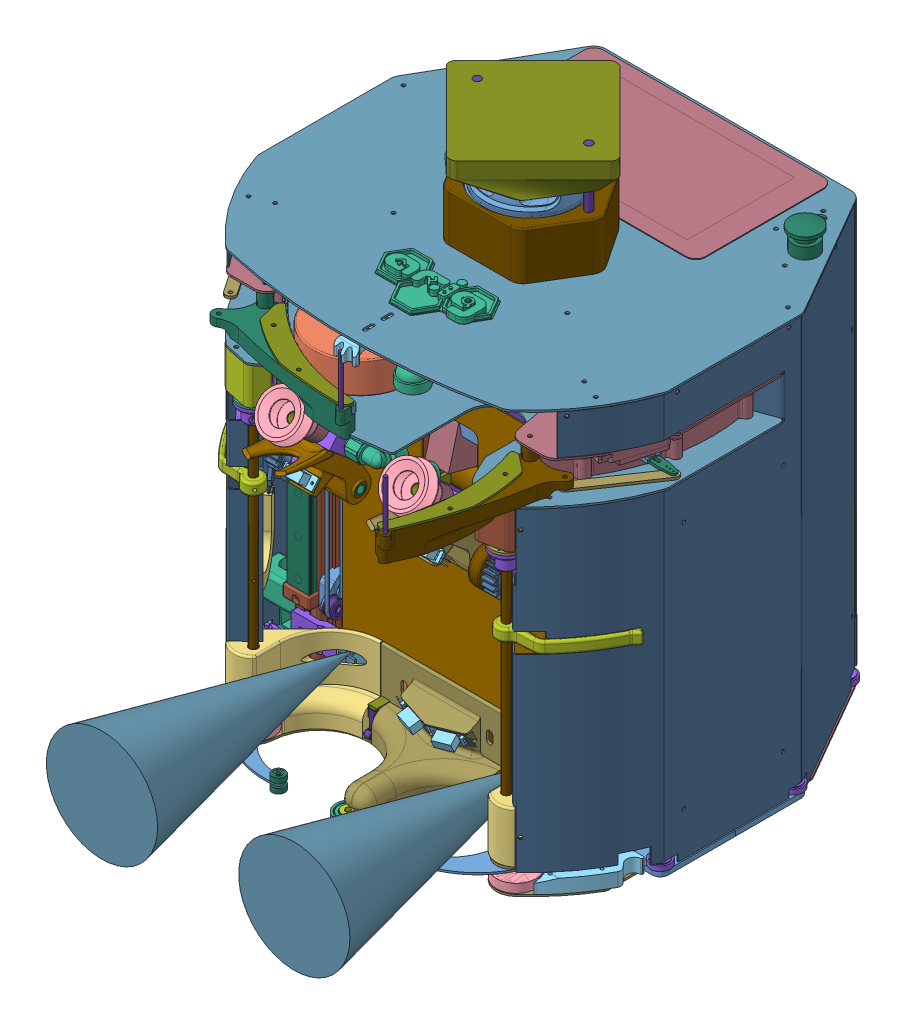
SolidWorks assembly 2019_Gros_robot, configuration Défaut. Lengths in mm.
Overall size (437.04 440.65 488.1).
582 component instances, 188 part files, 267 mates.
Components (placement in the parent):
- Robot2017_BaseRoulante-1: Robot2017_BaseRoulante [Défaut] at origin size (333 188.15 128.41)
  - Robot2015_BaseRoulante_piece01-1: Robot2015_BaseRoulante_piece01 [Défaut] at (0 7 0) size (330 4 120)
  - Robot2015_BaseRoulante_piece02-1: Robot2015_BaseRoulante_piece02 [Défaut] at (88 31 0) size (9.5 55 70)
  - Robot2015_BaseRoulante_piece02-2: Robot2015_BaseRoulante_piece02 [Défaut] at (55 31 0) x (-1 0 0) z (0 0 -1) size (9.5 55 70)
  - Robot2015_BaseRoulante_piece02-3: Robot2015_BaseRoulante_piece02 [Défaut] at (-55 31 0) size (9.5 55 70)
  - Robot2015_BaseRoulante_piece02-4: Robot2015_BaseRoulante_piece02 [Défaut] at (-88 31 0) x (-1 0 0) z (0 0 -1) size (9.5 55 70)
  - RoueMotrice-1: RoueMotrice [Défaut] at (109 -484.4772 -22.3565) x (0 -1 0) z (1 0 0) size (68.64 68.64 30)
    - Pneu-1: Pneu [Défaut] at (-515.4772 -22.3565 -15) size (64 64 30)
    - Jante-1: Jante [Défaut] at (-515.4772 -22.3565 15) x (-0.856398 -0.516316 0) z (0 0 1) size (50 50 30)
  - RoueMotrice-2: RoueMotrice [Défaut] at (-109 178.4325 494.4494) x (0 0.243951 0.969787) z (-1 0 0) size (68.64 68.64 30)
    - Pneu-1: Pneu [Défaut] at (-515.4772 -22.3565 -15) size (64 64 30)
    - Jante-1: Jante [Défaut] at (-515.4772 -22.3565 15) x (-0.856398 -0.516316 0) z (0 0 1) size (50 50 30)
  - Robot2015_BaseRoulante_piece03-1: Robot2015_BaseRoulante_piece03 [Défaut] at (117 31 0) size (67.5 12 14.69)
  - Robot2015_BaseRoulante_piece03-2: Robot2015_BaseRoulante_piece03 [Défaut] at (-117 31 0) x (-1 0 0) z (0 -0.777778 -0.62854) size (67.5 12 14.69)
  - roulement-1: roulement [Défaut] at (90 31 0) size (7 22 22)
  - roulement-2: roulement [Défaut] at (53 31 0) x (1 0 0) z (0 0.679013 0.734126) size (7 22 22)
  - roulement-3: roulement [Défaut] at (-53 31 0) x (1 0 0) z (0 0.679013 0.734126) size (7 22 22)
  - roulement-4: roulement [Défaut] at (-90 31 0) x (1 0 0) z (0 0.679013 0.734126) size (7 22 22)
  - Pignon XL037 pas5.08-1: Pignon XL037 pas5.08 [20 dents] at (67.65 31 0) x (1 0 0) z (0 -0.960015 0.27995) size (22 38 38)
  - Pignon XL037 pas5.08-2: Pignon XL037 pas5.08 [20 dents] at (67.65 149.9855 -19) x (-1 0 0) z (0 0.08811 -0.996111) size (22 38 38)
  - Robot2015_roulementAngle-1: Robot2015_roulementAngle [Défaut] at (158.5 13.75 53.5) size (16 9.5 16)
  - Robot2015_roulementAngle-2: Robot2015_roulementAngle [Défaut] at (158.5 13.75 -53.5) size (16 9.5 16)
  - Robot2015_roulementAngle-3: Robot2015_roulementAngle [Défaut] at (-158.5 13.75 53.5) size (16 9.5 16)
  - Robot2015_roulementAngle-4: Robot2015_roulementAngle [Défaut] at (-158.5 13.75 -53.5) size (16 9.5 16)
  - moteur-1: moteur [Défaut] at (48 149.9855 -19) x (0 -0.99965 -0.026437) z (1 0 0) size (42 42 188.5)
  - moteur-2: moteur [Défaut] at (-48 104.7937 -19) x (0 0.767621 0.640905) z (-1 0 0) size (42 42 188.5)
  - Pignon XL037 pas5.08-3: Pignon XL037 pas5.08 [20 dents] at (-67.65 31 0) x (-1 0 0) z (0 -0.781685 -0.623674) size (22 38 38)
  - Pignon XL037 pas5.08-4: Pignon XL037 pas5.08 [20 dents] at (-67.65 104.7937 -19) x (1 0 0) z (0 0.006752 0.999977) size (22 38 38)
  - Robot2015_profiléX20_01-1: Robot2015_profiléX20_01 [Défaut] at (-28 11 -40) x (0 0 -1) z (0 1 0) size (20 20 165)
  - Robot2015_profiléX20_01-2: Robot2015_profiléX20_01 [Défaut] at (48 11 -40) x (0 0 -1) z (0 1 0) size (20 20 165)
  - Robot2015_BaseRoulante_piece04-1: Robot2015_BaseRoulante_piece04 [Défaut] at (48 149.9855 -58) x (1 0 0) z (0 0 -1) size (3 50 44)
  - Robot2015_BaseRoulante_piece04-2: Robot2015_BaseRoulante_piece04 [Défaut] at (-51 104.7937 -58) x (1 0 0) z (0 0 -1) size (3 50 44)
  - Courroie1-5^Robot2017_BaseRoulante-1: Courroie1-5^Robot2017_BaseRoulante [Défaut] at (-67.65 104.7937 -19) x (0 0 -1) z (1 0 0) size (53.34 108.13 10) (virtual)
  - Courroie2-6^Robot2017_BaseRoulante-1: Courroie2-6^Robot2017_BaseRoulante [Défaut] at (67.65 149.9855 -19) x (0 0 1) z (-1 0 0) size (79.34 153.33 10) (virtual)
  - Robot2015_BaseRoulante_piece06-1: Robot2015_BaseRoulante_piece06 [Défaut] at (0 177.5 -61.5) size (256 20 20)
  - Igus_TK_04_09_Rail_L50-1: Igus_TK_04_09_Rail_L50 [Défaut] at (136 38.5 35) x (0 0 -1) z (1 0 0) size (9.6 50 6.3)
  - Igus_TK_04_09_coulisseau-1: Igus_TK_04_09_coulisseau [Défaut] at (136 101 35) x (0 0 -1) z (1 0 0) size (20 29 8.3)
  - Igus_TK_04_09_Rail_L50-2: Igus_TK_04_09_Rail_L50 [Défaut] at (136 38.5 -35) x (0 0 -1) z (1 0 0) size (9.6 50 6.3)
  - Igus_TK_04_09_coulisseau-2: Igus_TK_04_09_coulisseau [Défaut] at (136 101 -35) x (0 0 -1) z (1 0 0) size (20 29 8.3)
  - Igus_TK_04_09_Rail_L50-3: Igus_TK_04_09_Rail_L50 [Défaut] at (-136 38.5 35) x (0 0 1) z (-1 0 0) size (9.6 50 6.3)
  - Igus_TK_04_09_coulisseau-3: Igus_TK_04_09_coulisseau [Défaut] at (-136 101 35) x (0 0 1) z (-1 0 0) size (20 29 8.3)
  - Igus_TK_04_09_Rail_L50-4: Igus_TK_04_09_Rail_L50 [Défaut] at (-136 38.5 -35) x (0 0 1) z (-1 0 0) size (9.6 50 6.3)
  - Igus_TK_04_09_coulisseau-4: Igus_TK_04_09_coulisseau [Défaut] at (-136 101 -35) x (0 0 1) z (-1 0 0) size (20 29 8.3)
  - Kubler-05.2400.1212.1024-1: Kubler-05.2400.1212.1024 [fil a Gch] at (157 24 0) x (-1 0 0) z (0 0.34202 0.939693) size (31 88.25 62)
    - Kubler-05.2400.1212.1024-1: Kubler-05.2400.1212.1024 [Défaut] at origin size (31 36 24)
    - Kubler-rayon mini cable-1: Kubler-rayon mini cable [Défaut] at (25 -24 0) x (0 0 1) z (-1 0 0) size (52.25 52.25 4.5)
  - Kubler-05.2400.1212.1024-2: Kubler-05.2400.1212.1024 [fil a Drt] at (-157 24 0) x (1 0 0) z (0 -0.34202 -0.939693) size (31 88.25 62)
    - Kubler-05.2400.1212.1024-1: Kubler-05.2400.1212.1024 [Défaut] at origin size (31 36 24)
    - Kubler-rayon mini cable-1: Kubler-rayon mini cable [Défaut] at (25 -24 0) x (0 0 -1) z (1 0 0) size (52.25 52.25 4.5)
  - Robot2015_BaseRoulante_piece07-1: Robot2015_BaseRoulante_piece07 [Défaut] at (146 56.5 0) x (0 0 -1) z (1 0 0) size (93 50 1.5)
  - Robot2015_BaseRoulante_piece07-2: Robot2015_BaseRoulante_piece07 [Défaut] at (-146 56.5 0) x (0 0 1) z (-1 0 0) size (93 50 1.5)
  - Robot2015_BaseRoulante_piece08-1: Robot2015_BaseRoulante_piece08 [Défaut] at (51 38.5 30) size (85 55 10)
  - Robot2015_BaseRoulante_piece09-1: Robot2015_BaseRoulante_piece09 [Défaut] at (51 38.5 -30) x (1 0 0) z (0 0 -1) size (57 55 10)
  - Robot2015_BaseRoulante_piece09-2: Robot2015_BaseRoulante_piece09 [Défaut] at (-51 38.5 -30) x (-1 0 0) z (0 0 -1) size (57 55 10)
  - Robot2015_BaseRoulante_piece08-2: Robot2015_BaseRoulante_piece08 [Défaut] at (-51 38.5 30) x (-1 0 0) z (0 0 1) size (85 55 10)
  - Robot2015_BaseRoulante_piece10-1: Robot2015_BaseRoulante_piece10 [Défaut] at (155 24 0) x (-1 0 0) z (0 -0.545932 -0.837829) size (9 48 48)
  - Robot2015_BaseRoulante_piece10-2: Robot2015_BaseRoulante_piece10 [Défaut] at (-155 24 0) size (9 48 48)
  - Robot2015_BaseRoulante_piece11-1: Robot2015_BaseRoulante_piece11 [Défaut] at (79 66 0) x (0 0 -1) z (1 0 0) size (80 1.5 63)
  - Robot2015_BaseRoulante_piece11-2: Robot2015_BaseRoulante_piece11 [Défaut] at (-79 66 0) x (0 0 1) z (-1 0 0) size (80 1.5 63)
  - Robot2015_BaseRoulante_piece12-1: Robot2015_BaseRoulante_piece12 [Défaut] at (162 11 40) x (-1 0 0) z (0 0 -1) size (11.5 11.5 80)
  - Robot2015_BaseRoulante_piece12-2: Robot2015_BaseRoulante_piece12 [Défaut] at (-162 11 -40) size (11.5 11.5 80)
  - pignon renvoi 20 dents XL 2006-1: pignon renvoi 20 dents XL 2006 [Défaut] at (67.65 40 -45) x (1 0 0) z (0 0.474564 0.880221) size (9 32.34 32.34)
  - 20170402-1131-1: 20170402-1131 [Défaut] at (48 40 -45) x (0 0 -1) z (1 0 0) size (25 50 24.65)
  - 20170402-1229-1: 20170402-1229 [Défaut] at (73.15 40 -38.5) x (0 0 -1) z (1 0 0) size (25.5 30 9)
- batterieLIPO-1: batterieLIPO [Défaut] at (-65 97 -76) size (160 49 34)
- Robot2019_profiléX20_02-1: Robot2019_profiléX20_02 [Défaut] at (-110 276 40) x (0 0 1) z (0 -1 0) size (20 20 265)
- Robot2019_profiléX20_02-2: Robot2019_profiléX20_02 [Défaut] at (-110 276 -60) x (0 0 1) z (0 -1 0) size (20 20 265)
- Robot2019_profiléX20_02-3: Robot2019_profiléX20_02 [Défaut] at (130 276 40) x (0 0 1) z (0 -1 0) size (20 20 265)
- Robot2019_profiléX20_02-4: Robot2019_profiléX20_02 [Défaut] at (130 276 -60) x (0 0 1) z (0 -1 0) size (20 20 265)
- Robot2019_plaque bille porteuseAvant-1: Robot2019_plaque bille porteuseAvant [Défaut] at (0 5.5 0) size (300 1.5 120)
- Robot2019_plaque bille porteuse Arriere-1: Robot2019_plaque bille porteuse Arriere [Défaut] at (0 5.5 0) x (-1 0 0) z (0 0 -1) size (310 1.5 125)
- Robot2019_plaque du dessus-1: Robot2019_plaque du dessus [Défaut] at (0 276 0) size (330 1.5 300.96)
- APEM_A01ES_A0154B-1: APEM_A01ES_A0154B [Défaut] at (121.8383 345 -100) x (0.5 0 0.866025) z (-0.866025 0 0.5) size (24 61 24)
- bille porteuse-3: bille porteuse [Défaut] at (-111.446 0 -110) x (-0.5 0 -0.866025) z (0.866025 0 -0.5) size (49.64 21.5 47.15)
  - Robot2015_support bille porteuse-1: Robot2015_support bille porteuse [Défaut] at (0 9.5 0) size (49.64 12 45)
  - BillePorteuse-1: BillePorteuse [Défaut] at (0 7.5 0) x (0.947171 0 0.32073) z (0.32073 0 -0.947171) size (31 21.5 31)
- bille porteuse-4: bille porteuse [Défaut] at (111.446 0 -110) size (49.64 21.5 47.15)
  - Robot2015_support bille porteuse-1: Robot2015_support bille porteuse [Défaut] at (0 9.5 0) size (49.64 12 45)
  - BillePorteuse-1: BillePorteuse [Défaut] at (0 7.5 0) x (0.947171 0 0.32073) z (0.32073 0 -0.947171) size (31 21.5 31)
- pompe air 12v SFE-1: pompe air 12v SFE [Défaut] at (-20.6394 32 -38) size (38 60 92)
- rplidar-a2-1: rplidar-a2 [Défaut] at (-75 354.2861 -6.0269) x (0 0 -1) z (1 0 0) size (80.61 40.81 84.84)
- Robot2015_roulementAngle-1: Robot2015_roulementAngle [Défaut] at (100.765 9.75 -153.5) size (16 9.5 16)
- Robot2015_roulementAngle-2: Robot2015_roulementAngle [Défaut] at (-100.765 9.75 -153.5) size (16 9.5 16)
- 20180929-0119-1: 20180929-0119 [Défaut] at (0 277.5 0) x (-1 0 0) z (0 0 -1) size (291.8 157.5 260.35) (flexible)
  - Palet-1: Palet [Redium] at (-99.9974 12.7 0.7186) size (76.2 25.4 76.2)
  - Palet-2: Palet [Greenium] at (-49.3764 12.7 86.9596) size (76.2 25.4 76.2)
  - Palet-3: Palet [Redium] at (50.6211 12.7 86.241) size (76.2 25.4 76.2) (hidden)
  - Palet-4: Palet [Blueium] at (99.9974 12.7 -0.7186) x (0.648467 0 0.761243) z (-0.761243 0 0.648467) size (76.2 25.4 76.2)
  - Palet-5: Palet [Greenium] at (49.3764 12.7 -86.9596) x (0.321702 0 0.946841) z (-0.946841 0 0.321702) size (76.2 25.4 76.2)
  - Palet-6: Palet [Redium] at (-50.6211 12.7 -86.241) size (76.2 25.4 76.2) (hidden)
  - roulement-1: roulement [Défaut] at (81.9289 14.5 -48.09) x (0 -1 0) z (0.925744 0 -0.37815) size (7 22 22)
  - roulement-2: roulement [Défaut] at (-0.6827 14.5 -94.9975) x (0 -1 0) z (0.135385 0 -0.990793) size (7 22 22)
  - roulement-3: roulement [Défaut] at (-82.6116 14.5 -46.9075) x (0 -1 0) z (-0.79036 0 -0.612643) size (7 22 22)
  - roulement-4: roulement [Défaut] at (-81.9289 14.5 48.09) x (0 -1 0) z (-0.925744 0 0.37815) size (7 22 22)
  - roulement-5: roulement [Défaut] at (0.6827 14.5 94.9975) x (0 -1 0) z (-0.135385 0 0.990793) size (7 22 22)
  - roulement-6: roulement [Défaut] at (82.6116 14.5 46.9075) x (0 -1 0) z (0.79036 0 0.612643) size (7 22 22)
  - 20190528-1730-1: 20190528-1730 [Défaut] at (0 8.5 -22.5) x (0.926307 0 0.37677) z (-0.37677 0 0.926307) size (29.93 18 29.98)
  - 20181010-0239-1: 20181010-0239 [Défaut] at (0 8.5 0) x (0.853252 0 -0.521498) z (0.521498 0 0.853252) size (122.02 20.9 126.29)
  - PlaqueTounanteCarre94mm-1: PlaqueTounanteCarre94mm [Défaut] x (-0.707107 0 0.707107) z (-0.707107 0 -0.707107) size (115.6 8.5 115.6) (flexible)
    - PlaqueTounanteCarre94mm-1: PlaqueTounanteCarre94mm [Défaut] at origin size (94 8.25 94)
    - PlaqueTounanteCarre94mm-2: PlaqueTounanteCarre94mm [Défaut] at (0 8.5 0) x (-0.265754 0 -0.964041) z (-0.964041 0 0.265754) size (94 8.25 94)
  - 20190123-2151-1: 20190123-2151 [Défaut] at (0 16.5 0) x (-0.506211 0 -0.86241) z (0.86241 0 -0.506211) size (41.57 20.66 45)
  - 20190123-2208-1: 20190123-2208 [Défaut] at (81.9289 17.9 -48.09) x (-0.274765 0 -0.961511) z (-0.961511 0 0.274765) size (11.85 7.9 11.85)
  - 20190123-2208-2: 20190123-2208 [Défaut] at (-0.6827 17.9 -94.9975) x (-0.970076 0 -0.242802) z (-0.242802 0 0.970076) size (11.85 7.9 11.85)
  - 20190123-2208-3: 20190123-2208 [Défaut] at (-82.6116 17.9 -46.9075) x (-0.695311 0 0.718709) z (0.718709 0 0.695311) size (11.85 7.9 11.85)
  - 20190123-2208-4: 20190123-2208 [Défaut] at (-81.9289 17.9 48.09) x (0.274765 0 0.961511) z (0.961511 0 -0.274765) size (11.85 7.9 11.85)
  - 20190123-2208-5: 20190123-2208 [Défaut] at (0.6827 17.9 94.9975) x (0.970076 0 0.242802) z (0.242802 0 -0.970076) size (11.85 7.9 11.85)
  - 20190123-2208-6: 20190123-2208 [Défaut] at (82.6116 17.9 46.9075) x (0.695311 0 -0.718709) z (-0.718709 0 -0.695311) size (11.85 7.9 11.85)
  - 20190123-2151-2: 20190123-2151 [Défaut] at (0 16.5 0) x (-0.999974 0 0.007186) z (-0.007186 0 -0.999974) size (41.57 20.66 45)
  - 20190123-2151-3: 20190123-2151 [Défaut] at (0 16.5 0) x (-0.493764 0 0.869596) z (-0.869596 0 -0.493764) size (41.57 20.66 45)
  - 20190123-2151-4: 20190123-2151 [Défaut] at (0 16.5 0) x (0.506211 0 0.86241) z (-0.86241 0 0.506211) size (41.57 20.66 45)
  - 20190123-2151-5: 20190123-2151 [Défaut] at (0 16.5 0) x (0.999974 0 -0.007186) z (0.007186 0 0.999974) size (41.57 20.66 45)
  - 20190123-2151-6: 20190123-2151 [Défaut] at (0 16.5 0) x (0.493764 0 -0.869596) z (0.869596 0 0.493764) size (41.57 20.66 45)
  - 12v-silent-dc-motor-146rpm-encoder-desc-dime-1: 12v-silent-dc-motor-146rpm-encoder-desc-dime [Défaut] at (0 -2.5 -22.5) x (0 -1 0) z (-0.707107 0 -0.707107) size (123 36 36)
  - 20190124-0048-1: 20190124-0048 [Défaut] at (0 26.5 -22.5) x (0.37677 0 -0.926307) z (0.926307 0 0.37677) size (15 43 15)
  - NBB1,5-F79-E0-1: NBB1,5-F79-E0 [Défaut] at (43 30 0) x (1 0 0) z (0 0 -1) size (21 4.7 8)
  - 20190124-0123-1: 20190124-0123 [Défaut] at (47 32 -6.05) x (0 0 1) z (-1 0 0) size (19 4 16)
- 20181001-1750-1: 20181001-1750 [Défaut] at origin size (319.23 251.89 229.82)
  - Access_HS-645_BrasRondPetitModele-2: Access_HS-645_BrasRondPetitModele [Défaut] at (94 221.9292 85.221) x (0 0.153259 -0.988186) z (0 0.988186 0.153259) size (24 5 24)
  - Palet-1: Palet [Redium] at (50 270.0402 158.1056) x (1 0 0) z (0 0.766044 -0.642788) size (76.2 25.4 76.2) (hidden)
  - Servo_HS-805-BB-1: Servo_HS-805-BB [Défaut] at (-29 228 9) x (0 0.965926 -0.258819) z (0 0.258819 0.965926) size (82 65 29.5)
  - Access_HS-805_BrasRond-1: Access_HS-805_BrasRond [Défaut] at (-89 228 9) x (0 0 -1) z (0 1 0) size (39.6 8.5 39.6)
  - HIWIN_MGW09H 1 R 200 ZF H M SS_FILE-1: HIWIN_MGW09H 1 R 200 ZF H M SS_FILE [Défaut] at (-120 68 60) size (18 200 7)
  - HIWIN_MGW09H 1 R 200 ZF H M SS_FILE_1-1: HIWIN_MGW09H 1 R 200 ZF H M SS_FILE_1 [Défaut] at (-120 181.8091 60) size (30 51.3 9.1)
  - HIWIN_MGW09H 1 R 200 ZF H M SS_FILE-2: HIWIN_MGW09H 1 R 200 ZF H M SS_FILE [Défaut] at (120 68 60) size (18 200 7)
  - HIWIN_MGW09H 1 R 200 ZF H M SS_FILE_1-2: HIWIN_MGW09H 1 R 200 ZF H M SS_FILE_1 [Défaut] at (120 181.8091 60) size (30 51.3 9.1)
  - Galet_RainureU_4x13x7-1: Galet_RainureU_4x13x7 [Défaut] at (-95.5 68 62) x (1 0 0) z (0 1 0) size (7 13 13)
  - Galet_RainureU_4x13x7-2: Galet_RainureU_4x13x7 [Défaut] at (-95.5 188 50) x (1 0 0) z (0 1 0) size (7 13 13)
  - 20190123-2357-1: 20190123-2357 [Défaut] at (-98 228 9) x (1 0 0) z (0 0 -1) size (7 93 93)
  - Galet_RainureU_4x13x7-5: Galet_RainureU_4x13x7 [Défaut] at (-95.5 248 62) x (1 0 0) z (0 1 0) size (7 13 13)
  - 20190124-0203-1: 20190124-0203 [Défaut] at (-95.5 68 68) x (0 0 1) z (-1 0 0) size (104.52 211.5 2.55)
  - Servo_HS-805-BB-3: Servo_HS-805-BB [Défaut] at (29 228 9) x (0 0.965926 -0.258819) z (0 -0.258819 -0.965926) size (82 65 29.5)
  - SymétrieAccess_HS-805_BrasRond-3: SymétrieAccess_HS-805_BrasRond [Défaut] at (89 228 9) x (0 0 -1) z (0 -1 0) size (39.6 8.5 39.6)
  - 20190123-2357-3: 20190123-2357 [Défaut] at (98 228 9) x (-1 0 0) z (0 0 1) size (7 93 93)
  - Symétrie20190124-0203-2: Symétrie20190124-0203 [Défaut] at (95.5 68 68) x (0 0 1) z (-1 0 0) size (104.5 211.5 2.5)
  - Galet_RainureU_4x13x7-7: Galet_RainureU_4x13x7 [Défaut] at (95.5 248 62) x (-1 0 0) z (0 -1 0) size (7 13 13)
  - Galet_RainureU_4x13x7-8: Galet_RainureU_4x13x7 [Défaut] at (95.5 188 50) x (-1 0 0) z (0 -1 0) size (7 13 13)
  - Galet_RainureU_4x13x7-9: Galet_RainureU_4x13x7 [Défaut] at (95.5 68 62) x (-1 0 0) z (0 -1 0) size (7 13 13)
  - Ventouse_D33-1: Ventouse_D33 [Défaut] at (50 265.707 145.1629) x (1 0 0) z (0 0.766044 -0.642788) size (36.31 27 36.31)
  - 20170416-2304-1: 20170416-2304 [Défaut] at (54 209.1325 124.1007) x (1 0 0) z (0 0.642788 0.766044) size (30.6 16 70.4)
    - SupportCapteurPololu-1: SupportCapteurPololu [Défaut] at origin size (30 16 12.5) (hidden)
    - pololu gp2y0d805-1: pololu gp2y0d805 [Défaut] at (-14.5 -4.5 10.8) size (30.1 9 11.8)
    - faisceau pololu gp2y0d-1: faisceau pololu gp2y0d [5cm] at (-3.9 0 20.4) size (2 2 50) (hidden)
  - Legris_EQUERRE-OSCILLANTE_3159_06_10-1: Legris_EQUERRE-OSCILLANTE_3159_06_10 [Défaut] at (40 236.1388 109.9249) x (0 -0.296934 -0.954898) z (0 0.954898 -0.296934) size (28 34.3 15.01)
  - Legris_DouilleAnnelee_0934_10_10-1: Legris_DouilleAnnelee_0934_10_10 [Défaut] at (50 249.3159 125.6288) x (-0.990503 0.105326 -0.088379) z (0.137493 0.758769 -0.636683) size (15.24 32.5 12)
  - Legris_NourriceCroix_3312_00_10-1: Legris_NourriceCroix_3312_00_10 [Défaut] at (50 230.0104 115.0672) x (1 0 0) z (0 0.766044 -0.642788) size (30 30 16)
  - Legris_Bouchon_0220_10_00-1: Legris_Bouchon_0220_10_00 [Défaut] at (67.975 236.1388 109.9249) x (-1 0 0) z (0 -0.766044 0.642788) size (12.5 14 16.17)
  - 20181010-0238-2: 20181010-0238 [Défaut] at (78 201.6091 103) x (0 0.752597 -0.658481) z (0 -0.658481 -0.752597) size (29.93 18 29.98)
  - roulement_D8-D16-ep4-2: roulement_D8-D16-ep4 [Défaut] at (121.5 201.6091 103) x (1 0 0) z (0 -0.7977 0.603055) size (4 16 16)
  - 20190206-2329-1: 20190206-2329 [Défaut] at (50 265.707 145.1629) x (1 0 0) z (0 0.642788 0.766044) size (36.88 28.38 83.9)
  - 20190207-0044-1: 20190207-0044 [Défaut] at (50 254.1368 131.3741) x (0.792778 -0.466912 0.391786) z (0 -0.642788 -0.766044) size (18 18 13)
  - 20181010-0240-1: 20181010-0240 [Défaut] at (78.5 221.9292 85.221) x (0 0.752597 -0.658481) z (0 -0.658481 -0.752597) size (29.93 11 29.98)
  - 20190207-0111-1: 20190207-0111 [Défaut] at (33.5 201.6091 103) x (0 -0.866025 -0.5) z (-1 0 0) size (8 8 90)
  - roulement-1: roulement [Défaut] at (70 201.6091 103) size (7 22 22)
  - Servo_HS-645-MG_2-1: Servo_HS-645-MG_2 [Défaut] at (134.238 191.7032 75.442) x (0 0 1) z (0 -1 0) size (19.56 43.24 53.34)
  - 20190208-1431-1: 20190208-1431 [Défaut] at (66.5 181.6091 72) size (75 57 3)
  - 20190208-1506-1: 20190208-1506 [Défaut] at (109 238.6091 75) x (1 0 0) z (0 -1 0) size (76.02 43 57.11)
  - 20190209-0034-1: 20190209-0034 [Défaut] at (-110 68 50) x (0 0 1) z (1 0 0) size (24.5 25 12.5)
  - 20190209-0034-2: 20190209-0034 [Défaut] at (-110 248 50) x (0 0 1) z (1 0 0) size (24.5 25 12.5)
  - 20190209-0206-1: 20190209-0206 [Défaut] at (-110 200.5 50) x (0 0 -1) z (1 0 0) size (16 25 12.5)
  - 20190209-0206-2: 20190209-0206 [Défaut] at (110 200.5 50) x (0 0 1) z (-1 0 0) size (16 25 12.5)
  - 20190209-0034-3: 20190209-0034 [Défaut] at (110 248 50) x (0 0 1) z (-1 0 0) size (24.5 25 12.5)
  - 20190209-0034-4: 20190209-0034 [Défaut] at (110 68 50) x (0 0 1) z (-1 0 0) size (24.5 25 12.5)
  - 20190211-2116-1: 20190211-2116 [Défaut] at (148.047 126.5 67.5372) x (0.819152 0 0.573576) z (-0.573576 0 0.819152) size (12 87.35 50)
  - Igus_ChainePorteCable_ExtremiteA_modif2019-1: Igus_ChainePorteCable_ExtremiteA_modif2019 [Défaut] at (150.9141 126.5 69.5447) x (0 1 0) z (-0.573576 0 0.819152) size (26 36.15 16.39)
  - Igus_ChainePorteCable_ExtremiteB_modif2019-1: Igus_ChainePorteCable_ExtremiteB_modif2019 [Défaut] at (155.7489 256.7769 62.6133) x (0.099601 0.984808 -0.142244) z (-0.564863 0.173648 0.806707) size (25.74 12 18.61)
  - 20190212-2242-1: 20190212-2242 [Défaut] at (93.5 196.6091 72) size (8 24 3.9)
  - 20190212-2242-2: 20190212-2242 [Défaut] at (93.5 196.6091 64.2) x (1 0 0) z (0 0 -1) size (8 24 3.9)
  - 20190328-0013-1: 20190328-0013 [Défaut] at (73.5 201.6091 103) x (0 -0.835831 -0.548987) z (0 -0.548987 0.835831) size (14 4.5 14)
  - 20190208-1431-2: 20190208-1431 [Défaut] at (-66.5 181.6091 75) x (-1 0 0) z (0 0 -1) size (75 57 3)
  - Symétrie20190208-1506-2: Symétrie20190208-1506 [Défaut] at (-109 238.6091 75) x (-1 0 0) z (0 1 0) size (76.02 43 57.11)
  - Servo_HS-645-MG_2-2: Servo_HS-645-MG_2 [Défaut] at (-134.238 191.7032 95) x (0 0 -1) z (0 -1 0) size (19.56 43.24 53.34)
  - Access_HS-645_BrasRondPetitModele-3: Access_HS-645_BrasRondPetitModele [Défaut] at (-89 221.9292 85.221) x (0 -0.153259 0.988186) z (0 -0.988186 -0.153259) size (24 5 24)
  - 20181010-0240-2: 20181010-0240 [Défaut] at (-89.5 221.9292 85.221) x (0 0.752597 -0.658481) z (0 -0.658481 -0.752597) size (29.93 11 29.98)
  - 20181010-0238-3: 20181010-0238 [Défaut] at (-96 201.6091 103) x (0 0.752597 -0.658481) z (0 -0.658481 -0.752597) size (29.93 18 29.98)
  - 20190328-0013-2: 20190328-0013 [Défaut] at (-73.5 201.6091 103) x (0 -0.835831 -0.548987) z (0 0.548987 -0.835831) size (14 4.5 14)
  - 20190207-0111-2: 20190207-0111 [Défaut] at (-123.5 201.6091 103) x (0 -0.866025 -0.5) z (-1 0 0) size (8 8 90)
  - Symétrie20190206-2329-2: Symétrie20190206-2329 [Défaut] at (-50 265.707 145.1629) x (-1 0 0) z (0 -0.642788 -0.766044) size (36.88 28.38 83.9)
  - roulement_D8-D16-ep4-3: roulement_D8-D16-ep4 [Défaut] at (-121.5 201.6091 103) x (-1 0 0) z (0 0.7977 -0.603055) size (4 16 16)
  - roulement-2: roulement [Défaut] at (-70 201.6091 103) x (-1 0 0) z (0 0 -1) size (7 22 22)
  - 20170416-2304-2: 20170416-2304 [Défaut] at (-54 209.1325 124.1007) x (-1 0 0) z (0 0.642788 0.766044) size (30.6 16 70.4)
    - SupportCapteurPololu-1: SupportCapteurPololu [Défaut] at origin size (30 16 12.5) (hidden)
    - pololu gp2y0d805-1: pololu gp2y0d805 [Défaut] at (-14.5 -4.5 10.8) size (30.1 9 11.8)
    - faisceau pololu gp2y0d-1: faisceau pololu gp2y0d [5cm] at (-3.9 0 20.4) size (2 2 50) (hidden)
  - Legris_NourriceCroix_3312_00_10-2: Legris_NourriceCroix_3312_00_10 [Défaut] at (-50 242.2671 104.7826) x (-1 0 0) z (0 -0.766044 0.642788) size (30 30 16)
  - Legris_Bouchon_0220_10_00-2: Legris_Bouchon_0220_10_00 [Défaut] at (-67.975 236.1388 109.9249) x (1 0 0) z (0 0.766044 -0.642788) size (12.5 14 16.17)
  - SymétrieIgus_ChainePorteCable_ExtremiteA_modif2019-2: SymétrieIgus_ChainePorteCable_ExtremiteA_modif2019 [Défaut] at (-150.9141 126.5 69.5447) x (0 1 0) z (-0.573576 0 -0.819152) size (26 36.15 16.39)
  - 20190211-2116-2: 20190211-2116 [Défaut] at (-148.047 126.5 67.5372) x (0.819152 0 -0.573576) z (0.573576 0 0.819152) size (12 87.35 50)
  - Igus_ChainePorteCable_ExtremiteB_modif2019-2: Igus_ChainePorteCable_ExtremiteB_modif2019 [Défaut] at (-150.0148 256.7769 58.5983) x (-0.099601 0.984808 -0.142244) z (0.564863 0.173648 0.806707) size (25.74 12 18.61)
  - 20190207-0044-2: 20190207-0044 [Défaut] at (-50 254.1368 131.3741) x (0.792778 0.466912 -0.391786) z (0 -0.642788 -0.766044) size (18 18 13)
  - Ventouse_D33-2: Ventouse_D33 [Défaut] at (-50 265.707 145.1629) x (-1 0 0) z (0 -0.766044 0.642788) size (36.31 27 36.31)
  - Legris_DouilleAnnelee_0934_10_10-2: Legris_DouilleAnnelee_0934_10_10 [Défaut] at (-50 249.3159 125.6288) x (0.990503 0.105326 -0.088379) z (0.137493 -0.758769 0.636683) size (15.24 32.5 12)
  - Legris_EQUERRE-OSCILLANTE_3159_06_10-2: Legris_EQUERRE-OSCILLANTE_3159_06_10 [Défaut] at (-40 236.1388 109.9249) x (0 -0.296934 -0.954898) z (0 -0.954898 0.296934) size (28 34.3 15.01)
  - 20190409-2355-1: 20190409-2355 [Défaut] at (120 61 60) size (22 10 10.2)
  - 20190409-2355-2: 20190409-2355 [Défaut] at (120 275 60) x (-1 0 0) z (0 0 1) size (22 10 10.2)
  - 20190409-2355-3: 20190409-2355 [Défaut] at (-120 275 60) x (-1 0 0) z (0 0 1) size (22 10 10.2)
  - 20190409-2355-4: 20190409-2355 [Défaut] at (-120 61 60) size (22 10 10.2)
- 20181001-2148-1: 20181001-2148 [Défaut] at (-50 7 120) size (106 62 83)
- 20181002-0030-1: 20181002-0030 [Défaut] at (0 277.5 0) x (0.725374 0 0.688355) z (-0.688355 0 0.725374) size (312.09 32 306.03)
  - 20181002-0031-1: 20181002-0031 [Défaut] at origin size (146.08 16 151.84)
  - BagueRivetAIRBUS-1: BagueRivetAIRBUS [Défaut] at (141.5 15.8 0) x (0.352131 0 0.935951) z (0 1 0) size (6.8 6.8 5.6)
  - BagueRivetAIRBUS-2: BagueRivetAIRBUS [Défaut] at (141.3061 15.8 -7.4055) x (0.400633 0 0.916239) z (0 1 0) size (6.8 6.8 5.6)
  - BagueRivetAIRBUS-3: BagueRivetAIRBUS [Défaut] at (140.7248 15.8 -14.7908) x (0.448036 0 0.894016) z (0 1 0) size (6.8 6.8 5.6)
  - BagueRivetAIRBUS-4: BagueRivetAIRBUS [Défaut] at (139.7579 15.8 -22.1355) x (0.494211 0 0.869342) z (0 1 0) size (6.8 6.8 5.6)
  - BagueRivetAIRBUS-5: BagueRivetAIRBUS [Défaut] at (138.4079 15.8 -29.4195) x (0.539032 0 0.842286) z (0 1 0) size (6.8 6.8 5.6)
  - BagueRivetAIRBUS-6: BagueRivetAIRBUS [Défaut] at (136.6785 15.8 -36.6229) x (0.582375 0 0.812921) z (0 1 0) size (6.8 6.8 5.6)
  - BagueRivetAIRBUS-7: BagueRivetAIRBUS [Défaut] at (134.5745 15.8 -43.7259) x (0.624122 0 0.781327) z (0 1 0) size (6.8 6.8 5.6)
  - BagueRivetAIRBUS-8: BagueRivetAIRBUS [Défaut] at (132.1016 15.8 -50.7091) x (0.664158 0 0.747593) z (0 1 0) size (6.8 6.8 5.6)
  - BagueRivetAIRBUS-9: BagueRivetAIRBUS [Défaut] at (129.2667 15.8 -57.5532) x (0.702373 0 0.711809) z (0 1 0) size (6.8 6.8 5.6)
  - BagueRivetAIRBUS-10: BagueRivetAIRBUS [Défaut] at (126.0774 15.8 -64.2397) x (0.738664 0 0.674074) z (0 1 0) size (6.8 6.8 5.6)
  - BagueRivetAIRBUS-11: BagueRivetAIRBUS [Défaut] at (122.5426 15.8 -70.75) x (0.77293 0 0.634491) z (0 1 0) size (6.8 6.8 5.6)
  - BagueRivetAIRBUS-12: BagueRivetAIRBUS [Défaut] at (118.6719 15.8 -77.0664) x (0.805077 0 0.59317) z (0 1 0) size (6.8 6.8 5.6)
  - BagueRivetAIRBUS-13: BagueRivetAIRBUS [Défaut] at (114.4759 15.8 -83.1716) x (0.835018 0 0.550222) z (0 1 0) size (6.8 6.8 5.6)
  - BagueRivetAIRBUS-14: BagueRivetAIRBUS [Défaut] at (109.9662 15.8 -89.0488) x (0.86267 0 0.505767) z (0 1 0) size (6.8 6.8 5.6)
  - BagueRivetAIRBUS-15: BagueRivetAIRBUS [Défaut] at (105.155 15.8 -94.682) x (0.887958 0 0.459925) z (0 1 0) size (6.8 6.8 5.6)
  - BagueRivetAIRBUS-16: BagueRivetAIRBUS [Défaut] at (100.0556 15.8 -100.0556) x (0.910812 0 0.412822) z (0 1 0) size (6.8 6.8 5.6)
  - BagueRivetAIRBUS-17: BagueRivetAIRBUS [Défaut] at (94.682 15.8 -105.155) x (0.931169 0 0.364589) z (0 1 0) size (6.8 6.8 5.6)
  - BagueRivetAIRBUS-18: BagueRivetAIRBUS [Défaut] at (89.0488 15.8 -109.9662) x (0.948974 0 0.315355) z (0 1 0) size (6.8 6.8 5.6)
  - BagueRivetAIRBUS-19: BagueRivetAIRBUS [Défaut] at (83.1716 15.8 -114.4759) x (0.964178 0 0.265258) z (0 1 0) size (6.8 6.8 5.6)
  - BagueRivetAIRBUS-20: BagueRivetAIRBUS [Défaut] at (77.0664 15.8 -118.6719) x (0.976739 0 0.214433) z (0 1 0) size (6.8 6.8 5.6)
  - BagueRivetAIRBUS-21: BagueRivetAIRBUS [Défaut] at (70.75 15.8 -122.5426) x (0.986623 0 0.163021) z (0 1 0) size (6.8 6.8 5.6)
  - BagueRivetAIRBUS-22: BagueRivetAIRBUS [Défaut] at (64.2397 15.8 -126.0774) x (0.993802 0 0.111161) z (0 1 0) size (6.8 6.8 5.6)
  - BagueRivetAIRBUS-23: BagueRivetAIRBUS [Défaut] at (57.5532 15.8 -129.2667) x (0.998258 0 0.058997) z (0 1 0) size (6.8 6.8 5.6)
  - BagueRivetAIRBUS-24: BagueRivetAIRBUS [Défaut] at (50.7091 15.8 -132.1016) x (0.999978 0 0.006672) z (0 1 0) size (6.8 6.8 5.6)
  - BagueRivetAIRBUS-25: BagueRivetAIRBUS [Défaut] at (43.7259 15.8 -134.5745) x (0.998956 0 -0.045672) z (0 1 0) size (6.8 6.8 5.6)
  - BagueRivetAIRBUS-26: BagueRivetAIRBUS [Défaut] at (36.6229 15.8 -136.6785) x (0.995197 0 -0.097891) z (0 1 0) size (6.8 6.8 5.6)
  - BagueRivetAIRBUS-27: BagueRivetAIRBUS [Défaut] at (29.4195 15.8 -138.4079) x (0.98871 0 -0.149841) z (0 1 0) size (6.8 6.8 5.6)
  - BagueRivetAIRBUS-28: BagueRivetAIRBUS [Défaut] at (22.1355 15.8 -139.7579) x (0.979513 0 -0.201381) z (0 1 0) size (6.8 6.8 5.6)
  - BagueRivetAIRBUS-29: BagueRivetAIRBUS [Défaut] at (14.7908 15.8 -140.7248) x (0.967631 0 -0.252369) z (0 1 0) size (6.8 6.8 5.6)
  - BagueRivetAIRBUS-30: BagueRivetAIRBUS [Défaut] at (7.4055 15.8 -141.3061) x (0.953097 0 -0.302665) z (0 1 0) size (6.8 6.8 5.6)
  - 20181002-0031-2: 20181002-0031 [Défaut] at (0 32 0) x (0.052336 0 -0.99863) z (-0.99863 0 -0.052336) size (146.08 16 151.84)
  - 20181002-0031-3: 20181002-0031 [Défaut] x (0 0 -1) z (1 0 0) size (146.08 16 151.84)
  - 20181002-0031-4: 20181002-0031 [Défaut] x (-1 0 0) z (0 0 -1) size (146.08 16 151.84)
  - BagueRivetAIRBUS-91: BagueRivetAIRBUS [Défaut] at (0 15.8 -141.5) x (0.935951 0 -0.352131) z (0 1 0) size (6.8 6.8 5.6)
  - BagueRivetAIRBUS-92: BagueRivetAIRBUS [Défaut] at (-141.5 15.8 0) x (-0.352131 0 -0.935951) z (0 1 0) size (6.8 6.8 5.6)
  - BagueRivetAIRBUS-93: BagueRivetAIRBUS [Défaut] at (-7.4055 15.8 -141.3061) x (0.916239 0 -0.400633) z (0 1 0) size (6.8 6.8 5.6)
  - BagueRivetAIRBUS-94: BagueRivetAIRBUS [Défaut] at (-141.3061 15.8 7.4055) x (-0.400633 0 -0.916239) z (0 1 0) size (6.8 6.8 5.6)
  - BagueRivetAIRBUS-95: BagueRivetAIRBUS [Défaut] at (-29.4195 15.8 -138.4079) x (0.842286 0 -0.539032) z (0 1 0) size (6.8 6.8 5.6)
  - BagueRivetAIRBUS-96: BagueRivetAIRBUS [Défaut] at (-138.4079 15.8 29.4195) x (-0.539032 0 -0.842286) z (0 1 0) size (6.8 6.8 5.6)
  - BagueRivetAIRBUS-97: BagueRivetAIRBUS [Défaut] at (-22.1355 15.8 -139.7579) x (0.869342 0 -0.494211) z (0 1 0) size (6.8 6.8 5.6)
  - BagueRivetAIRBUS-98: BagueRivetAIRBUS [Défaut] at (-139.7579 15.8 22.1355) x (-0.494211 0 -0.869342) z (0 1 0) size (6.8 6.8 5.6)
  - BagueRivetAIRBUS-99: BagueRivetAIRBUS [Défaut] at (-36.6229 15.8 -136.6785) x (0.812921 0 -0.582375) z (0 1 0) size (6.8 6.8 5.6)
  - BagueRivetAIRBUS-100: BagueRivetAIRBUS [Défaut] at (-136.6785 15.8 36.6229) x (-0.582375 0 -0.812921) z (0 1 0) size (6.8 6.8 5.6)
  - BagueRivetAIRBUS-101: BagueRivetAIRBUS [Défaut] at (-43.7259 15.8 -134.5745) x (0.781327 0 -0.624122) z (0 1 0) size (6.8 6.8 5.6)
  - BagueRivetAIRBUS-102: BagueRivetAIRBUS [Défaut] at (-134.5745 15.8 43.7259) x (-0.624122 0 -0.781327) z (0 1 0) size (6.8 6.8 5.6)
  - BagueRivetAIRBUS-103: BagueRivetAIRBUS [Défaut] at (-14.7908 15.8 -140.7248) x (0.894016 0 -0.448036) z (0 1 0) size (6.8 6.8 5.6)
  - BagueRivetAIRBUS-104: BagueRivetAIRBUS [Défaut] at (-140.7248 15.8 14.7908) x (-0.448036 0 -0.894016) z (0 1 0) size (6.8 6.8 5.6)
  - BagueRivetAIRBUS-105: BagueRivetAIRBUS [Défaut] at (-50.7091 15.8 -132.1016) x (0.747593 0 -0.664158) z (0 1 0) size (6.8 6.8 5.6)
  - BagueRivetAIRBUS-106: BagueRivetAIRBUS [Défaut] at (-132.1016 15.8 50.7091) x (-0.664158 0 -0.747593) z (0 1 0) size (6.8 6.8 5.6)
  - BagueRivetAIRBUS-107: BagueRivetAIRBUS [Défaut] at (-64.2397 15.8 -126.0774) x (0.674074 0 -0.738664) z (0 1 0) size (6.8 6.8 5.6)
  - BagueRivetAIRBUS-108: BagueRivetAIRBUS [Défaut] at (-126.0774 15.8 64.2397) x (-0.738664 0 -0.674074) z (0 1 0) size (6.8 6.8 5.6)
  - BagueRivetAIRBUS-109: BagueRivetAIRBUS [Défaut] at (-70.75 15.8 -122.5426) x (0.634491 0 -0.77293) z (0 1 0) size (6.8 6.8 5.6)
  - BagueRivetAIRBUS-110: BagueRivetAIRBUS [Défaut] at (-122.5426 15.8 70.75) x (-0.77293 0 -0.634491) z (0 1 0) size (6.8 6.8 5.6)
  - BagueRivetAIRBUS-111: BagueRivetAIRBUS [Défaut] at (-100.0556 15.8 -100.0556) x (0.412822 0 -0.910812) z (0 1 0) size (6.8 6.8 5.6)
  - BagueRivetAIRBUS-112: BagueRivetAIRBUS [Défaut] at (-100.0556 15.8 100.0556) x (-0.910812 0 -0.412822) z (0 1 0) size (6.8 6.8 5.6)
  - BagueRivetAIRBUS-113: BagueRivetAIRBUS [Défaut] at (-122.5426 15.8 -70.75) x (0.163021 0 -0.986623) z (0 1 0) size (6.8 6.8 5.6)
  - BagueRivetAIRBUS-114: BagueRivetAIRBUS [Défaut] at (-70.75 15.8 122.5426) x (-0.986623 0 -0.163021) z (0 1 0) size (6.8 6.8 5.6)
  - BagueRivetAIRBUS-115: BagueRivetAIRBUS [Défaut] at (-94.682 15.8 -105.155) x (0.459925 0 -0.887958) z (0 1 0) size (6.8 6.8 5.6)
  - BagueRivetAIRBUS-116: BagueRivetAIRBUS [Défaut] at (-105.155 15.8 94.682) x (-0.887958 0 -0.459925) z (0 1 0) size (6.8 6.8 5.6)
  - BagueRivetAIRBUS-117: BagueRivetAIRBUS [Défaut] at (-129.2667 15.8 -57.5532) x (0.058997 0 -0.998258) z (0 1 0) size (6.8 6.8 5.6)
  - BagueRivetAIRBUS-118: BagueRivetAIRBUS [Défaut] at (-57.5532 15.8 129.2667) x (-0.998258 0 -0.058997) z (0 1 0) size (6.8 6.8 5.6)
  - BagueRivetAIRBUS-119: BagueRivetAIRBUS [Défaut] at (-136.6785 15.8 -36.6229) x (-0.097891 0 -0.995197) z (0 1 0) size (6.8 6.8 5.6)
  - BagueRivetAIRBUS-120: BagueRivetAIRBUS [Défaut] at (-36.6229 15.8 136.6785) x (-0.995197 0 0.097891) z (0 1 0) size (6.8 6.8 5.6)
  - BagueRivetAIRBUS-121: BagueRivetAIRBUS [Défaut] at (-141.3061 15.8 -7.4055) x (-0.302665 0 -0.953097) z (0 1 0) size (6.8 6.8 5.6)
  - BagueRivetAIRBUS-122: BagueRivetAIRBUS [Défaut] at (-7.4055 15.8 141.3061) x (-0.953097 0 0.302665) z (0 1 0) size (6.8 6.8 5.6)
  - BagueRivetAIRBUS-123: BagueRivetAIRBUS [Défaut] at (-77.0664 15.8 -118.6719) x (0.59317 0 -0.805077) z (0 1 0) size (6.8 6.8 5.6)
  - BagueRivetAIRBUS-124: BagueRivetAIRBUS [Défaut] at (-118.6719 15.8 77.0664) x (-0.805077 0 -0.59317) z (0 1 0) size (6.8 6.8 5.6)
  - BagueRivetAIRBUS-125: BagueRivetAIRBUS [Défaut] at (-118.6719 15.8 -77.0664) x (0.214433 0 -0.976739) z (0 1 0) size (6.8 6.8 5.6)
  - BagueRivetAIRBUS-126: BagueRivetAIRBUS [Défaut] at (-77.0664 15.8 118.6719) x (-0.976739 0 -0.214433) z (0 1 0) size (6.8 6.8 5.6)
  - BagueRivetAIRBUS-127: BagueRivetAIRBUS [Défaut] at (-139.7579 15.8 -22.1355) x (-0.201381 0 -0.979513) z (0 1 0) size (6.8 6.8 5.6)
  - BagueRivetAIRBUS-128: BagueRivetAIRBUS [Défaut] at (-22.1355 15.8 139.7579) x (-0.979513 0 0.201381) z (0 1 0) size (6.8 6.8 5.6)
  - BagueRivetAIRBUS-129: BagueRivetAIRBUS [Défaut] at (-57.5532 15.8 -129.2667) x (0.711809 0 -0.702373) z (0 1 0) size (6.8 6.8 5.6)
  - BagueRivetAIRBUS-130: BagueRivetAIRBUS [Défaut] at (-129.2667 15.8 57.5532) x (-0.702373 0 -0.711809) z (0 1 0) size (6.8 6.8 5.6)
  - BagueRivetAIRBUS-131: BagueRivetAIRBUS [Défaut] at (-105.155 15.8 -94.682) x (0.364589 0 -0.931169) z (0 1 0) size (6.8 6.8 5.6)
  - BagueRivetAIRBUS-132: BagueRivetAIRBUS [Défaut] at (-94.682 15.8 105.155) x (-0.931169 0 -0.364589) z (0 1 0) size (6.8 6.8 5.6)
  - BagueRivetAIRBUS-133: BagueRivetAIRBUS [Défaut] at (-126.0774 15.8 -64.2397) x (0.111161 0 -0.993802) z (0 1 0) size (6.8 6.8 5.6)
  - BagueRivetAIRBUS-134: BagueRivetAIRBUS [Défaut] at (-64.2397 15.8 126.0774) x (-0.993802 0 -0.111161) z (0 1 0) size (6.8 6.8 5.6)
  - BagueRivetAIRBUS-135: BagueRivetAIRBUS [Défaut] at (-109.9662 15.8 -89.0488) x (0.315355 0 -0.948974) z (0 1 0) size (6.8 6.8 5.6)
  - BagueRivetAIRBUS-136: BagueRivetAIRBUS [Défaut] at (-89.0488 15.8 109.9662) x (-0.948974 0 -0.315355) z (0 1 0) size (6.8 6.8 5.6)
  - BagueRivetAIRBUS-137: BagueRivetAIRBUS [Défaut] at (-132.1016 15.8 -50.7091) x (0.006672 0 -0.999978) z (0 1 0) size (6.8 6.8 5.6)
  - BagueRivetAIRBUS-138: BagueRivetAIRBUS [Défaut] at (-50.7091 15.8 132.1016) x (-0.999978 0 -0.006672) z (0 1 0) size (6.8 6.8 5.6)
  - BagueRivetAIRBUS-139: BagueRivetAIRBUS [Défaut] at (-138.4079 15.8 -29.4195) x (-0.149841 0 -0.98871) z (0 1 0) size (6.8 6.8 5.6)
  - BagueRivetAIRBUS-140: BagueRivetAIRBUS [Défaut] at (-29.4195 15.8 138.4079) x (-0.98871 0 0.149841) z (0 1 0) size (6.8 6.8 5.6)
  - BagueRivetAIRBUS-141: BagueRivetAIRBUS [Défaut] at (-134.5745 15.8 -43.7259) x (-0.045672 0 -0.998956) z (0 1 0) size (6.8 6.8 5.6)
  - BagueRivetAIRBUS-142: BagueRivetAIRBUS [Défaut] at (-43.7259 15.8 134.5745) x (-0.998956 0 0.045672) z (0 1 0) size (6.8 6.8 5.6)
  - BagueRivetAIRBUS-143: BagueRivetAIRBUS [Défaut] at (-140.7248 15.8 -14.7908) x (-0.252369 0 -0.967631) z (0 1 0) size (6.8 6.8 5.6)
  - BagueRivetAIRBUS-144: BagueRivetAIRBUS [Défaut] at (-14.7908 15.8 140.7248) x (-0.967631 0 0.252369) z (0 1 0) size (6.8 6.8 5.6)
  - BagueRivetAIRBUS-145: BagueRivetAIRBUS [Défaut] at (-83.1716 15.8 -114.4759) x (0.550222 0 -0.835018) z (0 1 0) size (6.8 6.8 5.6)
  - BagueRivetAIRBUS-146: BagueRivetAIRBUS [Défaut] at (-114.4759 15.8 83.1716) x (-0.835018 0 -0.550222) z (0 1 0) size (6.8 6.8 5.6)
  - BagueRivetAIRBUS-147: BagueRivetAIRBUS [Défaut] at (-89.0488 15.8 -109.9662) x (0.505767 0 -0.86267) z (0 1 0) size (6.8 6.8 5.6)
  - BagueRivetAIRBUS-148: BagueRivetAIRBUS [Défaut] at (-109.9662 15.8 89.0488) x (-0.86267 0 -0.505767) z (0 1 0) size (6.8 6.8 5.6)
  - BagueRivetAIRBUS-149: BagueRivetAIRBUS [Défaut] at (-114.4759 15.8 -83.1716) x (0.265258 0 -0.964178) z (0 1 0) size (6.8 6.8 5.6)
  - BagueRivetAIRBUS-150: BagueRivetAIRBUS [Défaut] at (-83.1716 15.8 114.4759) x (-0.964178 0 -0.265258) z (0 1 0) size (6.8 6.8 5.6)
  - 20181002-0031-5: 20181002-0031 [Défaut] at (0 32 0) x (-0.99863 0 -0.052336) z (-0.052336 0 0.99863) size (146.08 16 151.84)
  - 20181002-0031-6: 20181002-0031 [Défaut] at (0 32 0) x (-0.052336 0 0.99863) z (0.99863 0 0.052336) size (146.08 16 151.84)
- 20181002-0216-1: 20181002-0216 [Défaut] at (0 277.5 0) x (-0.688355 0 0.725374) z (-0.725374 0 -0.688355) size (81.93 62 112.21)
  - 20181002-0217-1: 20181002-0217 [Défaut] at origin size (81.17 33 112.21)
  - BagueRivetAIRBUS-1: BagueRivetAIRBUS [Défaut] at (141.5 15.8 0) x (0.352131 0 0.935951) z (0 1 0) size (6.8 6.8 5.6)
  - BagueRivetAIRBUS-2: BagueRivetAIRBUS [Défaut] at (141.3061 15.8 -7.4055) x (0.400633 0 0.916239) z (0 1 0) size (6.8 6.8 5.6)
  - BagueRivetAIRBUS-3: BagueRivetAIRBUS [Défaut] at (140.7248 15.8 -14.7908) x (0.448036 0 0.894016) z (0 1 0) size (6.8 6.8 5.6)
  - BagueRivetAIRBUS-4: BagueRivetAIRBUS [Défaut] at (139.7579 15.8 -22.1355) x (0.494211 0 0.869342) z (0 1 0) size (6.8 6.8 5.6)
  - BagueRivetAIRBUS-5: BagueRivetAIRBUS [Défaut] at (138.4079 15.8 -29.4195) x (0.539032 0 0.842286) z (0 1 0) size (6.8 6.8 5.6)
  - BagueRivetAIRBUS-6: BagueRivetAIRBUS [Défaut] at (136.6785 15.8 -36.6229) x (0.582375 0 0.812921) z (0 1 0) size (6.8 6.8 5.6)
  - BagueRivetAIRBUS-7: BagueRivetAIRBUS [Défaut] at (134.5745 15.8 -43.7259) x (0.624122 0 0.781327) z (0 1 0) size (6.8 6.8 5.6)
  - BagueRivetAIRBUS-8: BagueRivetAIRBUS [Défaut] at (132.1016 15.8 -50.7091) x (0.664158 0 0.747593) z (0 1 0) size (6.8 6.8 5.6)
  - BagueRivetAIRBUS-9: BagueRivetAIRBUS [Défaut] at (129.2667 15.8 -57.5532) x (0.702373 0 0.711809) z (0 1 0) size (6.8 6.8 5.6)
  - BagueRivetAIRBUS-10: BagueRivetAIRBUS [Défaut] at (126.0774 15.8 -64.2397) x (0.738664 0 0.674074) z (0 1 0) size (6.8 6.8 5.6)
  - BagueRivetAIRBUS-11: BagueRivetAIRBUS [Défaut] at (122.5426 15.8 -70.75) x (0.77293 0 0.634491) z (0 1 0) size (6.8 6.8 5.6)
  - BagueRivetAIRBUS-12: BagueRivetAIRBUS [Défaut] at (118.6719 15.8 -77.0664) x (0.805077 0 0.59317) z (0 1 0) size (6.8 6.8 5.6)
  - BagueRivetAIRBUS-13: BagueRivetAIRBUS [Défaut] at (114.4759 15.8 -83.1716) x (0.835018 0 0.550222) z (0 1 0) size (6.8 6.8 5.6)
  - BagueRivetAIRBUS-14: BagueRivetAIRBUS [Défaut] at (109.9662 15.8 -89.0488) x (0.86267 0 0.505767) z (0 1 0) size (6.8 6.8 5.6)
  - BagueRivetAIRBUS-15: BagueRivetAIRBUS [Défaut] at (105.155 15.8 -94.682) x (0.887958 0 0.459925) z (0 1 0) size (6.8 6.8 5.6)
  - 20190225-2246-1: 20190225-2246 [Défaut] at (-0.1569 19 -0.1746) x (-0.999824 0 -0.01876) z (0.01876 0 -0.999824) size (52.9 1.5 100.74)
  - 20190225-2359-1: 20190225-2359 [Défaut] at (110.3834 9 -100.2554) size (3 50 3)
- Symétrie20181002-0216-3: Symétrie20181002-0216 [Défaut] at (-34.7955 277.5 159.3024) x (0.946326 0 -0.323215) z (0.323215 0 0.946326) size (81.93 62 112.21)
  - Symétrie20181002-0217-1: Symétrie20181002-0217 [Défaut] at origin size (81.17 33 112.21)
  - SymétrieBagueRivetAIRBUS-1: SymétrieBagueRivetAIRBUS [Défaut] at (141.5 15.8 0) x (0.352131 0 -0.935951) z (0 -1 0) size (6.8 6.8 5.6)
  - SymétrieBagueRivetAIRBUS-2: SymétrieBagueRivetAIRBUS [Défaut] at (141.3061 12.8 7.4055) x (0.400633 0 -0.916239) z (0 -1 0) size (6.8 6.8 5.6)
  - SymétrieBagueRivetAIRBUS-3: SymétrieBagueRivetAIRBUS [Défaut] at (140.7248 12.8 14.7908) x (0.448036 0 -0.894016) z (0 -1 0) size (6.8 6.8 5.6)
  - SymétrieBagueRivetAIRBUS-4: SymétrieBagueRivetAIRBUS [Défaut] at (139.7579 12.8 22.1355) x (0.494211 0 -0.869342) z (0 -1 0) size (6.8 6.8 5.6)
  - SymétrieBagueRivetAIRBUS-5: SymétrieBagueRivetAIRBUS [Défaut] at (138.4079 12.8 29.4195) x (0.539032 0 -0.842286) z (0 -1 0) size (6.8 6.8 5.6)
  - SymétrieBagueRivetAIRBUS-6: SymétrieBagueRivetAIRBUS [Défaut] at (136.6785 12.8 36.6229) x (0.582375 0 -0.812921) z (0 -1 0) size (6.8 6.8 5.6)
  - SymétrieBagueRivetAIRBUS-7: SymétrieBagueRivetAIRBUS [Défaut] at (134.5745 12.8 43.7259) x (0.624122 0 -0.781327) z (0 -1 0) size (6.8 6.8 5.6)
  - SymétrieBagueRivetAIRBUS-8: SymétrieBagueRivetAIRBUS [Défaut] at (132.1016 12.8 50.7091) x (0.664158 0 -0.747593) z (0 -1 0) size (6.8 6.8 5.6)
  - SymétrieBagueRivetAIRBUS-9: SymétrieBagueRivetAIRBUS [Défaut] at (129.2667 12.8 57.5532) x (0.702373 0 -0.711809) z (0 -1 0) size (6.8 6.8 5.6)
  - SymétrieBagueRivetAIRBUS-10: SymétrieBagueRivetAIRBUS [Défaut] at (126.0774 12.8 64.2397) x (0.738664 0 -0.674074) z (0 -1 0) size (6.8 6.8 5.6)
  - SymétrieBagueRivetAIRBUS-11: SymétrieBagueRivetAIRBUS [Défaut] at (122.5426 12.8 70.75) x (0.77293 0 -0.634491) z (0 -1 0) size (6.8 6.8 5.6)
  - SymétrieBagueRivetAIRBUS-12: SymétrieBagueRivetAIRBUS [Défaut] at (118.6719 12.8 77.0664) x (0.805077 0 -0.59317) z (0 -1 0) size (6.8 6.8 5.6)
  - SymétrieBagueRivetAIRBUS-13: SymétrieBagueRivetAIRBUS [Défaut] at (114.4759 12.8 83.1716) x (0.835018 0 -0.550222) z (0 -1 0) size (6.8 6.8 5.6)
  - SymétrieBagueRivetAIRBUS-14: SymétrieBagueRivetAIRBUS [Défaut] at (109.9662 12.8 89.0488) x (0.86267 0 -0.505767) z (0 -1 0) size (6.8 6.8 5.6)
  - SymétrieBagueRivetAIRBUS-15: SymétrieBagueRivetAIRBUS [Défaut] at (105.155 12.8 94.682) x (0.887958 0 -0.459925) z (0 -1 0) size (6.8 6.8 5.6)
  - 20190225-2359-1: 20190225-2359 [Défaut] at (110.3834 9 100.2554) size (3 50 3)
  - 20190225-2246-1: 20190225-2246 [Défaut] at (0 20.5 0) x (-0.999848 0 0.017414) z (0.017414 0 0.999848) size (52.9 1.5 100.74)
